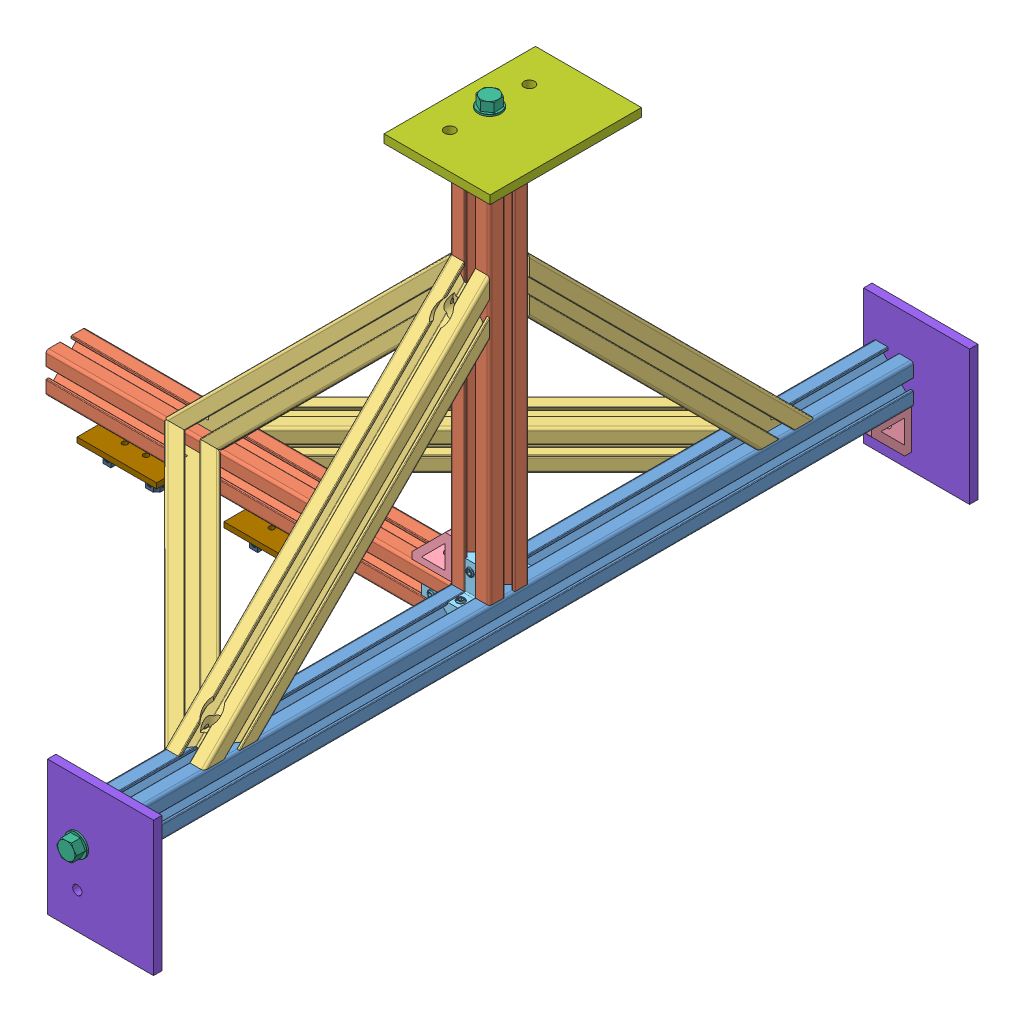
SolidWorks assembly AASY Leg Mount, configuration Default. Lengths in mm.
Overall size (377.3 391.65 639).
27 component instances, 10 part files, 75 mates.
Components (placement in the parent):
- 5537T737_ALUMINUM T-SLOTTED FRAMING EXTRUSION-1: 5537T737_ALUMINUM T-SLOTTED FRAMING EXTRUSION [5537T737] at (243.2576 328.5857 452.5216) size (30 30 609.6)
- 5537T736_ALUMINUM T-SLOTTED FRAMING EXTRUSION-1: 5537T736_ALUMINUM T-SLOTTED FRAMING EXTRUSION [5537T736] at (243.2576 495.9856 452.5216) x (1 0 0) z (0 -1 0) size (30 30 304.8)
- 5537T604_ALUMINUM T-SLOTTED FRAMING EXTRUSION-1: 5537T604_ALUMINUM T-SLOTTED FRAMING EXTRUSION [5537T604] at (131.1011 440.7422 452.5216) x (0 0 -1) z (0.707107 0.707107 0) size (30 30 304.8)
- 5537T736_ALUMINUM T-SLOTTED FRAMING EXTRUSION-2: 5537T736_ALUMINUM T-SLOTTED FRAMING EXTRUSION [5537T736] at (75.8576 328.5857 452.5216) x (0 0 -1) z (1 0 0) size (30 30 304.8)
- 5537T604_ALUMINUM T-SLOTTED FRAMING EXTRUSION-2: 5537T604_ALUMINUM T-SLOTTED FRAMING EXTRUSION [5537T604] at (243.2576 440.7422 340.3652) x (1 0 0) z (0 0.707107 0.707107) size (30 30 304.8)
- 5537T604_ALUMINUM T-SLOTTED FRAMING EXTRUSION-3: 5537T604_ALUMINUM T-SLOTTED FRAMING EXTRUSION [5537T604] at (131.1011 328.5857 564.6781) x (0 -1 0) z (-0.707107 0 -0.707107) size (30 30 304.8)
- 5537T604_ALUMINUM T-SLOTTED FRAMING EXTRUSION-4: 5537T604_ALUMINUM T-SLOTTED FRAMING EXTRUSION [5537T604] at (243.2576 440.7422 564.6781) x (-1 0 0) z (0 0.707107 -0.707107) size (30 30 304.8)
- 5537T604_ALUMINUM T-SLOTTED FRAMING EXTRUSION-5: 5537T604_ALUMINUM T-SLOTTED FRAMING EXTRUSION [5537T604] at (131.1011 328.5857 340.3652) x (0 1 0) z (-0.707107 0 0.707107) size (30 30 304.8)
- 5537T536_T-SLOTTED FRAMING-1: 5537T536_T-SLOTTED FRAMING [5537T536] at (243.2576 648.3856 437.5216) x (0 0 -1) z (-1 0 0) size (30 30 27)
- 5537T536_T-SLOTTED FRAMING-2: 5537T536_T-SLOTTED FRAMING [5537T536] at (243.2576 313.5858 757.3216) x (0 0 -1) z (-1 0 0) size (30 30 27)
- 5537T536_T-SLOTTED FRAMING-3: 5537T536_T-SLOTTED FRAMING [5537T536] at (243.2576 648.3856 467.5216) x (0 0 1) z (1 0 0) size (30 30 27)
- 5537T536_T-SLOTTED FRAMING-4: 5537T536_T-SLOTTED FRAMING [5537T536] at (243.2576 313.5858 147.7216) x (0 -1 0) z (-1 0 0) size (30 30 27)
- 5537T316_ALUMINUM T-SLOTTED FRAMING EXTRUSION-2: 5537T316_ALUMINUM T-SLOTTED FRAMING EXTRUSION [5537T316] at (236.5151 328.5857 445.7792) x (0 -1 0) z (0 0 -1) size (15.8 30 21)
- 5537T316_ALUMINUM T-SLOTTED FRAMING EXTRUSION-3: 5537T316_ALUMINUM T-SLOTTED FRAMING EXTRUSION [5537T316] at (243.2576 335.3282 445.7792) x (-1 0 0) z (0 0 -1) size (15.8 30 21)
- 5537T316_ALUMINUM T-SLOTTED FRAMING EXTRUSION-4: 5537T316_ALUMINUM T-SLOTTED FRAMING EXTRUSION [5537T316] at (236.5151 328.5857 459.2641) x (0 1 0) z (0 0 1) size (15.8 30 21)
- 5537T316_ALUMINUM T-SLOTTED FRAMING EXTRUSION-5: 5537T316_ALUMINUM T-SLOTTED FRAMING EXTRUSION [5537T316] at (243.2576 335.3282 459.2641) size (15.8 30 21)
- 5537T536_T-SLOTTED FRAMING-5: 5537T536_T-SLOTTED FRAMING [5537T536] at (228.2576 343.5856 452.5216) x (-1 0 0) z (0 0 -1) size (30 30 27)
- 94209A341_THREAD-FORMING SCREWS FOR SOFT METAL-1: 94209A341_THREAD-FORMING SCREWS FOR SOFT METAL [94209A341] at (243.2576 328.5857 141.3716) x (-0.923728 -0.383049 0) z (0 0 -1) size (17 17 38.35)
- 94209A341_THREAD-FORMING SCREWS FOR SOFT METAL-2: 94209A341_THREAD-FORMING SCREWS FOR SOFT METAL [94209A341] at (243.2576 328.5857 763.6716) x (-0.021369 0.999772 0) z (0 0 1) size (17 17 38.35)
- McMasterBackPlate-1: McMasterBackPlate [Default] at (220.7576 648.3856 509.6716) x (0 0 -1) z (0 1 0) size (114.3 80 6.35)
- McMasterSidePlate-1: McMasterSidePlate [Default] at (220.7576 373.0357 147.7216) x (0 -1 0) z (0 0 -1) size (101.6 80 6.35)
- 94209A341_THREAD-FORMING SCREWS FOR SOFT METAL-3: 94209A341_THREAD-FORMING SCREWS FOR SOFT METAL [94209A341] at (243.2576 654.7356 452.5216) x (0.56381 0 0.825904) z (0 1 0) size (17 17 38.35)
- McMasterSidePlate-2: McMasterSidePlate [Default] at (220.7576 373.0357 763.6716) x (0 -1 0) z (0 0 -1) size (101.6 80 6.35)
- 5537T386_ALUMINUM T-SLOTTED FRAMING EXTRUSION-1: 5537T386_ALUMINUM T-SLOTTED FRAMING EXTRUSION [5537T386] at (72.7429 311.5858 422.5216) x (1 0 0) z (0 -1 0) size (60 60 4)
- 5537T386_ALUMINUM T-SLOTTED FRAMING EXTRUSION-2: 5537T386_ALUMINUM T-SLOTTED FRAMING EXTRUSION [5537T386] at (-38.0571 311.5858 422.5216) x (1 0 0) z (0 -1 0) size (60 60 4)
- 1201-0043-0002-1: 1201-0043-0002 [Default] at (-8.0571 309.5858 452.5216) x (-1 0 0) z (0 0 1) size (43.01 12.01 43.01)
- 1201-0043-0002-2: 1201-0043-0002 [Default] at (102.7429 309.5858 452.5216) x (1 0 0) z (0 0 -1) size (43.01 12.01 43.01)
Mates (geometry in assembly coordinates):
- Coincident1: coincident anti-aligned: plane of 5537T737_ALUMINUM T-SLOTTED FRAMING EXTRUSION-1 through (238.7576 343.5856 757.3216) normal (0 1 0); plane of 5537T736_ALUMINUM T-SLOTTED FRAMING EXTRUSION-1 through (257.7575 343.5856 448.0216) normal (0 -1 0)
- Width1: width anti-aligned: plane of 5537T737_ALUMINUM T-SLOTTED FRAMING EXTRUSION-1 through (257.7575 324.0857 757.3216) normal (0 0 1); plane of 5537T737_ALUMINUM T-SLOTTED FRAMING EXTRUSION-1 through (257.7575 324.0857 147.7216) normal (0 0 -1); plane of 5537T736_ALUMINUM T-SLOTTED FRAMING EXTRUSION-1 through (247.7576 343.5856 437.5217) normal (0 0 -1); plane of 5537T736_ALUMINUM T-SLOTTED FRAMING EXTRUSION-1 through (256.2575 343.5856 467.5216) normal (0 0 1)
- Coincident2: coincident aligned: plane of 5537T737_ALUMINUM T-SLOTTED FRAMING EXTRUSION-1 through (258.2575 333.0857 757.3216) normal (1 0 0); plane of 5537T736_ALUMINUM T-SLOTTED FRAMING EXTRUSION-1 through (258.2575 343.5856 457.0216) normal (1 0 0)
- Coincident3: coincident anti-aligned: plane of 5537T736_ALUMINUM T-SLOTTED FRAMING EXTRUSION-1 through (228.2576 343.5856 465.5216) normal (-1 0 0); plane of 5537T604_ALUMINUM T-SLOTTED FRAMING EXTRUSION-1 through (228.2576 516.6856 467.5216) normal (1 0 0)
- Coincident4: coincident aligned: plane of 5537T736_ALUMINUM T-SLOTTED FRAMING EXTRUSION-1 through (238.7576 343.5856 467.5216) normal (0 0 1); plane of 5537T604_ALUMINUM T-SLOTTED FRAMING EXTRUSION-1 through (229.6718 557.6976 467.5216) normal (0 0 1)
- Coincident6: coincident anti-aligned: plane of 5537T737_ALUMINUM T-SLOTTED FRAMING EXTRUSION-1 through (238.7576 343.5856 757.3216) normal (0 1 0); plane of 5537T604_ALUMINUM T-SLOTTED FRAMING EXTRUSION-2 through (228.2576 343.5856 264.4218) normal (0 -1 0)
- Coincident7: coincident anti-aligned: plane of 5537T736_ALUMINUM T-SLOTTED FRAMING EXTRUSION-1 through (247.7576 343.5856 437.5217) normal (0 0 -1); plane of 5537T604_ALUMINUM T-SLOTTED FRAMING EXTRUSION-2 through (228.2576 516.6856 437.5217) normal (0 0 1)
- Coincident8: coincident aligned: plane of 5537T736_ALUMINUM T-SLOTTED FRAMING EXTRUSION-1 through (258.2575 343.5856 439.5217) normal (1 0 0); plane of 5537T604_ALUMINUM T-SLOTTED FRAMING EXTRUSION-2 through (258.2575 551.6872 444.9463) normal (1 0 0)
- Coincident9: coincident anti-aligned: plane of 5537T736_ALUMINUM T-SLOTTED FRAMING EXTRUSION-1 through (256.2575 343.5856 467.5216) normal (0 0 1); plane of 5537T604_ALUMINUM T-SLOTTED FRAMING EXTRUSION-4 through (258.2575 516.6856 467.5216) normal (0 0 -1)
- Coincident10: coincident aligned: plane of 5537T736_ALUMINUM T-SLOTTED FRAMING EXTRUSION-1 through (258.2575 343.5856 457.0216) normal (1 0 0); plane of 5537T604_ALUMINUM T-SLOTTED FRAMING EXTRUSION-4 through (258.2575 557.6976 466.1074) normal (1 0 0)
- Coincident11: coincident anti-aligned: plane of 5537T737_ALUMINUM T-SLOTTED FRAMING EXTRUSION-1 through (238.7576 343.5856 757.3216) normal (0 1 0); plane of 5537T604_ALUMINUM T-SLOTTED FRAMING EXTRUSION-4 through (258.2575 343.5856 640.6215) normal (0 -1 0)
- Coincident12: coincident anti-aligned: plane of 5537T737_ALUMINUM T-SLOTTED FRAMING EXTRUSION-1 through (228.2576 341.5857 757.3216) normal (-1 0 0); plane of 5537T736_ALUMINUM T-SLOTTED FRAMING EXTRUSION-2 through (228.2576 324.0857 438.0217) normal (1 0 0)
- Coincident13: coincident aligned: plane of 5537T736_ALUMINUM T-SLOTTED FRAMING EXTRUSION-1 through (238.7576 343.5856 467.5216) normal (0 0 1); plane of 5537T736_ALUMINUM T-SLOTTED FRAMING EXTRUSION-2 through (228.2576 341.5857 467.5216) normal (0 0 1)
- Coincident14: coincident aligned: plane of 5537T737_ALUMINUM T-SLOTTED FRAMING EXTRUSION-1 through (230.2576 313.5858 757.3216) normal (0 -1 0); plane of 5537T736_ALUMINUM T-SLOTTED FRAMING EXTRUSION-2 through (228.2576 313.5858 465.5216) normal (0 -1 0)
- Coincident15: coincident anti-aligned: plane of 5537T736_ALUMINUM T-SLOTTED FRAMING EXTRUSION-2 through (228.2576 341.5857 467.5216) normal (0 0 1); plane of 5537T604_ALUMINUM T-SLOTTED FRAMING EXTRUSION-3 through (55.1577 343.5856 467.5216) normal (0 0 -1)
- Coincident16: coincident anti-aligned: plane of 5537T737_ALUMINUM T-SLOTTED FRAMING EXTRUSION-1 through (228.2576 324.0857 757.3216) normal (-1 0 0); plane of 5537T604_ALUMINUM T-SLOTTED FRAMING EXTRUSION-3 through (228.2576 343.5856 640.6215) normal (1 0 0)
- Coincident17: coincident aligned: plane of 5537T736_ALUMINUM T-SLOTTED FRAMING EXTRUSION-2 through (228.2576 313.5858 465.5216) normal (0 -1 0); plane of 5537T604_ALUMINUM T-SLOTTED FRAMING EXTRUSION-3 through (20.156 313.5858 460.097) normal (0 -1 0)
- Coincident18: coincident anti-aligned: plane of 5537T604_ALUMINUM T-SLOTTED FRAMING EXTRUSION-1 through (55.1577 343.5856 467.5216) normal (0 -1 0); plane of 5537T736_ALUMINUM T-SLOTTED FRAMING EXTRUSION-2 through (228.2576 343.5856 439.5217) normal (0 1 0)
- Coincident19: coincident anti-aligned: plane of 5537T737_ALUMINUM T-SLOTTED FRAMING EXTRUSION-1 through (228.2576 324.0857 757.3216) normal (-1 0 0); plane of 5537T604_ALUMINUM T-SLOTTED FRAMING EXTRUSION-5 through (228.2576 313.5858 264.4218) normal (1 0 0)
- Coincident20: coincident anti-aligned: plane of 5537T736_ALUMINUM T-SLOTTED FRAMING EXTRUSION-2 through (228.2576 315.5858 437.5217) normal (0 0 -1); plane of 5537T604_ALUMINUM T-SLOTTED FRAMING EXTRUSION-5 through (55.1577 313.5858 437.5217) normal (0 0 1)
- Coincident21: coincident aligned: plane of 5537T736_ALUMINUM T-SLOTTED FRAMING EXTRUSION-2 through (228.2576 313.5858 448.0216) normal (0 -1 0); plane of 5537T604_ALUMINUM T-SLOTTED FRAMING EXTRUSION-5 through (14.1457 313.5858 438.9359) normal (0 -1 0)
- Width2: width anti-aligned: plane of 5537T736_ALUMINUM T-SLOTTED FRAMING EXTRUSION-1 through (228.2576 343.5856 448.0216) normal (-1 0 0); plane of 5537T736_ALUMINUM T-SLOTTED FRAMING EXTRUSION-1 through (258.2575 343.5856 439.5217) normal (1 0 0); plane of 5537T536_T-SLOTTED FRAMING-1 through (256.7576 648.3856 437.5216) normal (1 0 0); plane of 5537T536_T-SLOTTED FRAMING-1 through (229.7576 648.3856 437.5216) normal (-1 0 0)
- Width3: width anti-aligned: plane of 5537T736_ALUMINUM T-SLOTTED FRAMING EXTRUSION-1 through (228.2576 343.5856 465.5216) normal (-1 0 0); plane of 5537T736_ALUMINUM T-SLOTTED FRAMING EXTRUSION-1 through (258.2575 343.5856 457.0216) normal (1 0 0); plane of 5537T536_T-SLOTTED FRAMING-2 through (229.7576 313.5858 757.3216) normal (-1 0 0); plane of 5537T536_T-SLOTTED FRAMING-2 through (256.7576 313.5858 757.3216) normal (1 0 0)
- Width4: width anti-aligned: plane of 5537T737_ALUMINUM T-SLOTTED FRAMING EXTRUSION-1 through (228.2576 341.5857 757.3216) normal (-1 0 0); plane of 5537T737_ALUMINUM T-SLOTTED FRAMING EXTRUSION-1 through (258.2575 333.0857 757.3216) normal (1 0 0); plane of 5537T536_T-SLOTTED FRAMING-4 through (256.7576 313.5858 147.7216) normal (1 0 0); plane of 5537T536_T-SLOTTED FRAMING-4 through (229.7576 313.5858 147.7216) normal (-1 0 0)
- Width5: width anti-aligned: plane of 5537T737_ALUMINUM T-SLOTTED FRAMING EXTRUSION-1 through (228.2576 324.0857 757.3216) normal (-1 0 0); plane of 5537T737_ALUMINUM T-SLOTTED FRAMING EXTRUSION-1 through (258.2575 315.5858 757.3216) normal (1 0 0); plane of 5537T536_T-SLOTTED FRAMING-3 through (256.7576 648.3856 467.5216) normal (1 0 0); plane of 5537T536_T-SLOTTED FRAMING-3 through (229.7576 648.3856 467.5216) normal (-1 0 0)
- Coincident23: coincident aligned: plane of 5537T737_ALUMINUM T-SLOTTED FRAMING EXTRUSION-1 through (257.7575 324.0857 757.3216) normal (0 0 1); plane of 5537T536_T-SLOTTED FRAMING-2 through (256.7576 313.5858 757.3216) normal (0 0 1)
- Coincident24: coincident anti-aligned: plane of 5537T737_ALUMINUM T-SLOTTED FRAMING EXTRUSION-1 through (247.7576 313.5858 757.3216) normal (0 -1 0); plane of 5537T536_T-SLOTTED FRAMING-2 through (256.7576 313.5858 757.3216) normal (0 1 0)
- Coincident25: coincident anti-aligned: plane of 5537T737_ALUMINUM T-SLOTTED FRAMING EXTRUSION-1 through (230.2576 313.5858 757.3216) normal (0 -1 0); plane of 5537T536_T-SLOTTED FRAMING-4 through (256.7576 313.5858 147.7216) normal (0 1 0)
- Coincident26: coincident aligned: plane of 5537T737_ALUMINUM T-SLOTTED FRAMING EXTRUSION-1 through (257.7575 324.0857 147.7216) normal (0 0 -1); plane of 5537T536_T-SLOTTED FRAMING-4 through (256.7576 313.5858 147.7216) normal (0 0 -1)
- Coincident27: coincident anti-aligned: plane of 5537T736_ALUMINUM T-SLOTTED FRAMING EXTRUSION-1 through (230.2576 343.5856 437.5217) normal (0 0 -1); plane of 5537T536_T-SLOTTED FRAMING-1 through (256.7576 648.3856 437.5216) normal (0 0 1)
- Coincident28: coincident aligned: plane of 5537T736_ALUMINUM T-SLOTTED FRAMING EXTRUSION-1 through (257.7575 648.3856 448.0216) normal (0 1 0); plane of 5537T536_T-SLOTTED FRAMING-1 through (256.7576 648.3856 437.5216) normal (0 1 0)
- Coincident29: coincident anti-aligned: plane of 5537T736_ALUMINUM T-SLOTTED FRAMING EXTRUSION-1 through (238.7576 343.5856 467.5216) normal (0 0 1); plane of 5537T536_T-SLOTTED FRAMING-3 through (229.7576 648.3856 467.5216) normal (0 0 -1)
- Coincident30: coincident aligned: plane of 5537T736_ALUMINUM T-SLOTTED FRAMING EXTRUSION-1 through (257.7575 648.3856 448.0216) normal (0 1 0); plane of 5537T536_T-SLOTTED FRAMING-3 through (229.7576 648.3856 467.5216) normal (0 1 0)
- Coincident31: coincident anti-aligned: plane of 5537T736_ALUMINUM T-SLOTTED FRAMING EXTRUSION-2 through (228.2576 320.8532 465.2641) normal (0 0 -1); plane of 5537T316_ALUMINUM T-SLOTTED FRAMING EXTRUSION-4 through (222.5151 324.6857 465.2641) normal (0 0 1)
- Coincident32: coincident anti-aligned: plane of 5537T737_ALUMINUM T-SLOTTED FRAMING EXTRUSION-1 through (230.5151 320.8532 757.3216) normal (1 0 0); plane of 5537T316_ALUMINUM T-SLOTTED FRAMING EXTRUSION-4 through (230.5151 320.6857 461.2641) normal (-1 0 0)
- Width6: width anti-aligned: plane of 5537T737_ALUMINUM T-SLOTTED FRAMING EXTRUSION-1 through (238.7576 343.5856 757.3216) normal (0 1 0); plane of 5537T737_ALUMINUM T-SLOTTED FRAMING EXTRUSION-1 through (230.2576 313.5858 757.3216) normal (0 -1 0); plane of 5537T316_ALUMINUM T-SLOTTED FRAMING EXTRUSION-4 through (230.5151 324.6857 461.2641) normal (0 -1 0); plane of 5537T316_ALUMINUM T-SLOTTED FRAMING EXTRUSION-4 through (230.5151 332.4857 461.2641) normal (0 1 0)
- Coincident33: coincident anti-aligned: plane of 5537T737_ALUMINUM T-SLOTTED FRAMING EXTRUSION-1 through (230.5151 333.0857 757.3216) normal (1 0 0); plane of 5537T316_ALUMINUM T-SLOTTED FRAMING EXTRUSION-2 through (230.5151 336.4857 443.7792) normal (-1 0 0)
- Coincident34: coincident anti-aligned: plane of 5537T736_ALUMINUM T-SLOTTED FRAMING EXTRUSION-2 through (228.2576 336.3182 439.7792) normal (0 0 1); plane of 5537T316_ALUMINUM T-SLOTTED FRAMING EXTRUSION-2 through (222.5151 332.4857 439.7792) normal (0 0 -1)
- Width7: width anti-aligned: plane of 5537T736_ALUMINUM T-SLOTTED FRAMING EXTRUSION-2 through (228.2576 343.5856 439.5217) normal (0 1 0); plane of 5537T736_ALUMINUM T-SLOTTED FRAMING EXTRUSION-2 through (228.2576 313.5858 448.0216) normal (0 -1 0); plane of 5537T316_ALUMINUM T-SLOTTED FRAMING EXTRUSION-2 through (222.5151 320.6857 439.7792) normal (0 -1 0); plane of 5537T316_ALUMINUM T-SLOTTED FRAMING EXTRUSION-2 through (222.5151 336.4857 439.7792) normal (0 1 0)
- Width8: width aligned: plane of 5537T736_ALUMINUM T-SLOTTED FRAMING EXTRUSION-1 through (258.2575 343.5856 439.5217) normal (1 0 0); plane of 5537T736_ALUMINUM T-SLOTTED FRAMING EXTRUSION-1 through (228.2576 343.5856 448.0216) normal (-1 0 0); plane of 5537T316_ALUMINUM T-SLOTTED FRAMING EXTRUSION-5 through (247.1576 341.3282 461.2641) normal (1 0 0); plane of 5537T316_ALUMINUM T-SLOTTED FRAMING EXTRUSION-5 through (239.3576 341.3282 461.2641) normal (-1 0 0)
- Coincident36: coincident anti-aligned: plane of 5537T316_ALUMINUM T-SLOTTED FRAMING EXTRUSION-5 through (247.1576 349.3282 465.2641) normal (0 0 1); plane of 5537T736_ALUMINUM T-SLOTTED FRAMING EXTRUSION-1 through (247.7576 343.5856 465.2641) normal (0 0 -1)
- Coincident37: coincident anti-aligned: plane of 5537T737_ALUMINUM T-SLOTTED FRAMING EXTRUSION-1 through (247.7576 341.3282 757.3216) normal (0 -1 0); plane of 5537T316_ALUMINUM T-SLOTTED FRAMING EXTRUSION-5 through (251.1576 341.3282 461.2641) normal (0 1 0)
- Width9: width anti-aligned: plane of 5537T316_ALUMINUM T-SLOTTED FRAMING EXTRUSION-3 through (239.3576 341.3282 443.7792) normal (-1 0 0); plane of 5537T316_ALUMINUM T-SLOTTED FRAMING EXTRUSION-3 through (247.1576 341.3282 443.7792) normal (1 0 0); plane of 5537T736_ALUMINUM T-SLOTTED FRAMING EXTRUSION-1 through (228.2576 343.5856 448.0216) normal (-1 0 0); plane of 5537T736_ALUMINUM T-SLOTTED FRAMING EXTRUSION-1 through (258.2575 343.5856 439.5217) normal (1 0 0)
- Coincident38: coincident anti-aligned: plane of 5537T736_ALUMINUM T-SLOTTED FRAMING EXTRUSION-1 through (238.7576 343.5856 439.7792) normal (0 0 1); plane of 5537T316_ALUMINUM T-SLOTTED FRAMING EXTRUSION-3 through (239.3576 349.3282 439.7792) normal (0 0 -1)
- Coincident39: coincident anti-aligned: plane of 5537T737_ALUMINUM T-SLOTTED FRAMING EXTRUSION-1 through (235.525 341.3282 757.3216) normal (0 -1 0); plane of 5537T316_ALUMINUM T-SLOTTED FRAMING EXTRUSION-3 through (235.3576 341.3282 443.7792) normal (0 1 0)
- Width10: width anti-aligned: plane of 5537T736_ALUMINUM T-SLOTTED FRAMING EXTRUSION-2 through (228.2576 341.5857 467.5216) normal (0 0 1); plane of 5537T736_ALUMINUM T-SLOTTED FRAMING EXTRUSION-2 through (228.2576 333.0857 437.5217) normal (0 0 -1); plane of 5537T536_T-SLOTTED FRAMING-5 through (228.2576 343.5856 466.0216) normal (0 0 1); plane of 5537T536_T-SLOTTED FRAMING-5 through (228.2576 343.5856 439.0216) normal (0 0 -1)
- Coincident40: coincident anti-aligned: plane of 5537T736_ALUMINUM T-SLOTTED FRAMING EXTRUSION-2 through (228.2576 343.5856 457.0216) normal (0 1 0); plane of 5537T536_T-SLOTTED FRAMING-5 through (228.2576 343.5856 466.0216) normal (0 -1 0)
- Coincident41: coincident anti-aligned: plane of 5537T736_ALUMINUM T-SLOTTED FRAMING EXTRUSION-1 through (228.2576 343.5856 448.0216) normal (-1 0 0); plane of 5537T536_T-SLOTTED FRAMING-5 through (228.2576 343.5856 466.0216) normal (1 0 0)
- Concentric1: concentric aligned: cylinder of 5537T737_ALUMINUM T-SLOTTED FRAMING EXTRUSION-1 through (243.2576 328.5857 757.3216) axis (0 0 -1) radius 3.53; cylinder of 94209A341_THREAD-FORMING SCREWS FOR SOFT METAL-2 through (243.2576 328.5857 765.0076) axis (0 0 -1) radius 8.5
- Concentric3: concentric anti-aligned: cylinder of 5537T737_ALUMINUM T-SLOTTED FRAMING EXTRUSION-1 through (243.2576 328.5857 757.3216) axis (0 0 -1) radius 3.53; cylinder of 94209A341_THREAD-FORMING SCREWS FOR SOFT METAL-1 through (243.2576 328.5857 140.0356) axis (0 0 1) radius 8.5
- Concentric4: concentric anti-aligned: cylinder of 5537T737_ALUMINUM T-SLOTTED FRAMING EXTRUSION-1 through (243.2576 328.5857 757.3216) axis (0 0 -1) radius 3.53; cylinder of McMasterSidePlate-1 through (243.2576 328.5857 141.3716) axis (0 0 1) radius 4
- Concentric5: concentric anti-aligned: cylinder of 5537T536_T-SLOTTED FRAMING-4 through (243.2576 298.5858 162.7216) axis (0 0 -1) radius 3.5; cylinder of McMasterSidePlate-1 through (243.2576 298.5857 141.3716) axis (0 0 1) radius 3.5
- Coincident42: coincident anti-aligned: plane of 5537T536_T-SLOTTED FRAMING-4 through (256.7576 313.5858 147.7216) normal (0 0 -1); plane of McMasterSidePlate-1 through (220.7576 373.0357 147.7216) normal (0 0 1)
- Coincident43: coincident anti-aligned: plane of 94209A341_THREAD-FORMING SCREWS FOR SOFT METAL-1 through (235.4059 325.3298 141.3716) normal (0 0 1); plane of McMasterSidePlate-1 through (220.7576 373.0357 141.3716) normal (0 0 -1)
- Concentric6: concentric anti-aligned: cylinder of 5537T736_ALUMINUM T-SLOTTED FRAMING EXTRUSION-1 through (243.2576 343.5856 452.5216) axis (0 1 0) radius 3.53; cylinder of McMasterBackPlate-1 through (243.2576 654.7356 452.5216) axis (0 -1 0) radius 4
- Concentric9: concentric anti-aligned: cylinder of 5537T536_T-SLOTTED FRAMING-3 through (243.2576 633.3856 482.5216) axis (0 1 0) radius 3.5; cylinder of McMasterBackPlate-1 through (243.2576 654.7356 482.5216) axis (0 -1 0) radius 4
- Concentric10: concentric anti-aligned: cylinder of 5537T536_T-SLOTTED FRAMING-1 through (243.2576 633.3856 422.5216) axis (0 1 0) radius 3.5; cylinder of McMasterBackPlate-1 through (243.2576 654.7356 422.5216) axis (0 -1 0) radius 4
- Coincident44: coincident anti-aligned: plane of 5537T736_ALUMINUM T-SLOTTED FRAMING EXTRUSION-1 through (257.7575 648.3856 448.0216) normal (0 1 0); plane of McMasterBackPlate-1 through (220.7576 648.3856 509.6716) normal (0 -1 0)
- Concentric11: concentric aligned: cylinder of McMasterBackPlate-1 through (243.2576 654.7356 452.5216) axis (0 -1 0) radius 4; cylinder of 94209A341_THREAD-FORMING SCREWS FOR SOFT METAL-3 through (243.2576 656.0716 452.5216) axis (0 -1 0) radius 8.5
- Coincident45: coincident anti-aligned: plane of McMasterBackPlate-1 through (220.7576 654.7356 509.6716) normal (0 1 0); plane of 94209A341_THREAD-FORMING SCREWS FOR SOFT METAL-3 through (248.0499 654.7356 459.5418) normal (0 -1 0)
- Concentric12: concentric aligned: circle of 5537T737_ALUMINUM T-SLOTTED FRAMING EXTRUSION-1; cylinder of McMasterSidePlate-2 through (243.2576 328.5857 757.3216) axis (0 0 1) radius 4
- Concentric13: concentric aligned: cylinder of 5537T536_T-SLOTTED FRAMING-2 through (243.2576 298.5858 742.3216) axis (0 0 1) radius 3.5; cylinder of McMasterSidePlate-2 through (243.2576 298.5857 757.3216) axis (0 0 1) radius 3.5
- Coincident46: coincident anti-aligned: plane of 94209A341_THREAD-FORMING SCREWS FOR SOFT METAL-2 through (243.0759 337.0838 763.6716) normal (0 0 -1); plane of McMasterSidePlate-2 through (220.7576 373.0357 763.6716) normal (0 0 1)
- Coincident47: coincident anti-aligned: plane of 5537T737_ALUMINUM T-SLOTTED FRAMING EXTRUSION-1 through (257.7575 324.0857 757.3216) normal (0 0 1); plane of McMasterSidePlate-2 through (220.7576 373.0357 757.3216) normal (0 0 -1)
- Width11: width aligned: plane of 5537T386_ALUMINUM T-SLOTTED FRAMING EXTRUSION-1 through (132.7429 309.5858 422.5216) normal (0 0 -1); plane of 5537T386_ALUMINUM T-SLOTTED FRAMING EXTRUSION-1 through (132.7429 309.5858 482.5216) normal (0 0 1); plane of 5537T736_ALUMINUM T-SLOTTED FRAMING EXTRUSION-2 through (228.2576 315.5858 437.5217) normal (0 0 -1); plane of 5537T736_ALUMINUM T-SLOTTED FRAMING EXTRUSION-2 through (228.2576 324.0857 467.5216) normal (0 0 1)
- Coincident48: coincident anti-aligned: plane of 5537T736_ALUMINUM T-SLOTTED FRAMING EXTRUSION-2 through (228.2576 313.5858 465.5216) normal (0 -1 0); plane of 5537T386_ALUMINUM T-SLOTTED FRAMING EXTRUSION-1 through (72.7429 313.5858 422.5216) normal (0 1 0)
- Width12: width anti-aligned: plane of 5537T386_ALUMINUM T-SLOTTED FRAMING EXTRUSION-2 through (21.9429 309.5858 422.5216) normal (0 0 -1); plane of 5537T386_ALUMINUM T-SLOTTED FRAMING EXTRUSION-2 through (21.9429 309.5858 482.5216) normal (0 0 1); plane of 5537T736_ALUMINUM T-SLOTTED FRAMING EXTRUSION-2 through (228.2576 324.0857 467.5216) normal (0 0 1); plane of 5537T736_ALUMINUM T-SLOTTED FRAMING EXTRUSION-2 through (228.2576 315.5858 437.5217) normal (0 0 -1)
- Coincident49: coincident anti-aligned: plane of 5537T736_ALUMINUM T-SLOTTED FRAMING EXTRUSION-2 through (228.2576 313.5858 448.0216) normal (0 -1 0); plane of 5537T386_ALUMINUM T-SLOTTED FRAMING EXTRUSION-2 through (-38.0571 313.5858 422.5216) normal (0 1 0)
- Distance1: distance = 50.8 mm anti-aligned: plane of 5537T386_ALUMINUM T-SLOTTED FRAMING EXTRUSION-2 through (21.9429 309.5858 482.5216) normal (1 0 0); plane of 5537T386_ALUMINUM T-SLOTTED FRAMING EXTRUSION-1 through (72.7429 309.5858 422.5216) normal (-1 0 0)
- Coincident50: coincident anti-aligned: plane of 5537T386_ALUMINUM T-SLOTTED FRAMING EXTRUSION-2 through (-38.0571 309.5858 422.5216) normal (0 -1 0); plane of 1201-0043-0002-1 through (-8.0571 309.5858 452.5216) normal (0 1 0)
- Width13: width aligned: plane of 5537T386_ALUMINUM T-SLOTTED FRAMING EXTRUSION-2 through (21.9429 309.5858 422.5216) normal (0 0 -1); plane of 1201-0043-0002-1 through (21.9429 309.5858 482.5216) normal (0 0 1); plane of 5537T386_ALUMINUM T-SLOTTED FRAMING EXTRUSION-2 through (-8.0571 318.7782 431.0216) normal (0 0 -1); plane of 1201-0043-0002-1 through (-8.0571 318.7782 474.0216) normal (0 0 1)
- Width14: width aligned: plane of 5537T386_ALUMINUM T-SLOTTED FRAMING EXTRUSION-2 through (-38.0571 309.5858 422.5216) normal (-1 0 0); plane of 1201-0043-0002-1 through (21.9429 309.5858 482.5216) normal (1 0 0); plane of 5537T386_ALUMINUM T-SLOTTED FRAMING EXTRUSION-2 through (-27.0571 305.5858 452.5216) normal (-1 0 0); plane of 1201-0043-0002-1 through (10.9429 305.5858 452.5216) normal (1 0 0)
- Coincident51: coincident anti-aligned: plane of 5537T386_ALUMINUM T-SLOTTED FRAMING EXTRUSION-1 through (72.7429 309.5858 422.5216) normal (0 -1 0); plane of 1201-0043-0002-2 through (102.7429 309.5858 452.5216) normal (0 1 0)
- Width15: width aligned: plane of 5537T386_ALUMINUM T-SLOTTED FRAMING EXTRUSION-1 through (132.7429 309.5858 482.5216) normal (0 0 1); plane of 1201-0043-0002-2 through (132.7429 309.5858 422.5216) normal (0 0 -1); plane of 5537T386_ALUMINUM T-SLOTTED FRAMING EXTRUSION-1 through (102.7429 318.7782 474.0216) normal (0 0 1); plane of 1201-0043-0002-2 through (102.7429 318.7782 431.0216) normal (0 0 -1)
- Width16: width aligned: plane of 5537T386_ALUMINUM T-SLOTTED FRAMING EXTRUSION-1 through (132.7429 309.5858 482.5216) normal (1 0 0); plane of 1201-0043-0002-2 through (72.7429 309.5858 422.5216) normal (-1 0 0); plane of 5537T386_ALUMINUM T-SLOTTED FRAMING EXTRUSION-1 through (121.7429 305.5858 452.5216) normal (1 0 0); plane of 1201-0043-0002-2 through (83.7429 305.5858 452.5216) normal (-1 0 0)
